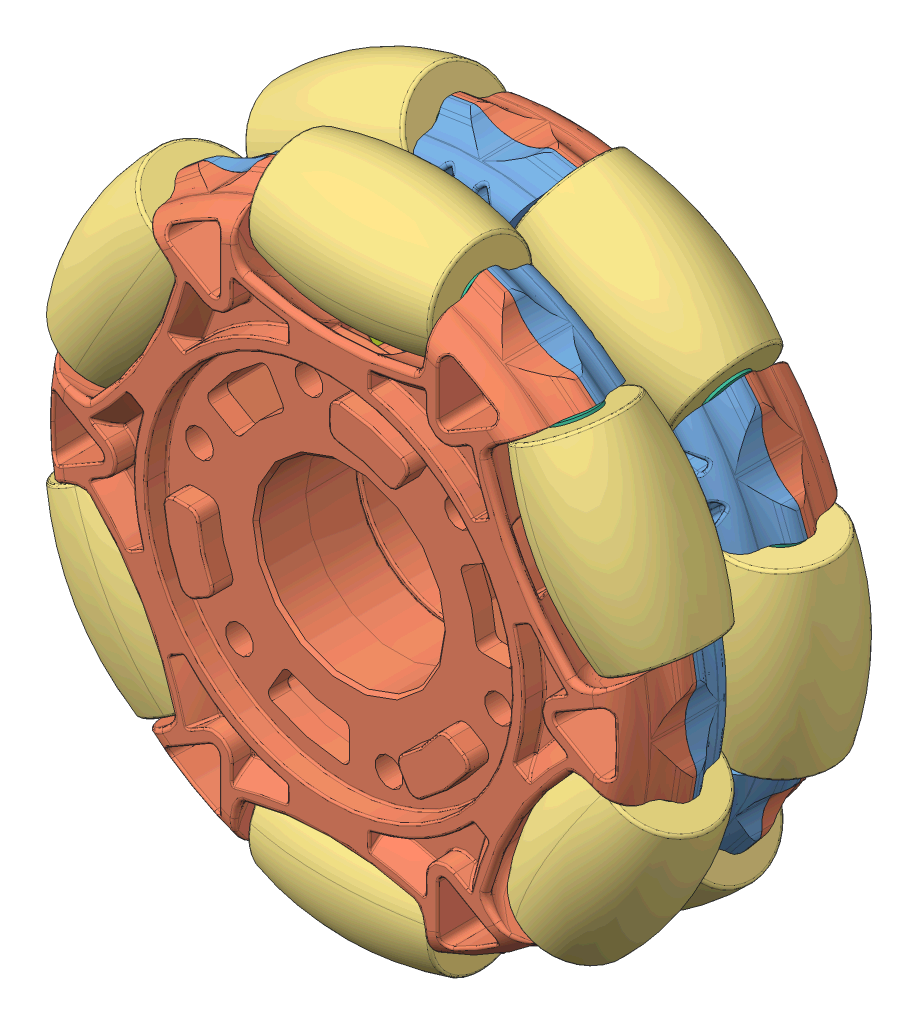
SolidWorks assembly 4_Omni-Directional_Wheel_v2_276-6194, configuration Default. Lengths in mm.
Overall size (126.87 125.33 42.82).
82 component instances, 8 part files, 0 mates.
Components (placement in the parent):
- 4_Omni-Directional_Wheel_v2_276-6194(2)-1: 4_Omni-Directional_Wheel_v2_276-6194(2) [Default] at origin size (126.87 125.33 42.82)
  - 217-6194-002 Rev5-1: 217-6194-002 Rev5 [Default] at origin size (94.42 94.42 19.26)
  - 217-6194-003 Rev8-1: 217-6194-003 Rev8 [Default] at (0 0 9.525) size (94.42 90.2 19.97)
  - 217-6194-003 Rev8-2: 217-6194-003 Rev8 [Default] at (0 0 -9.525) x (-0.866025 0.5 0) z (0 0 -1) size (94.42 90.2 19.97)
  - 217-6194-001 Rev3-1: 217-6194-001 Rev3 [Default] at (0 -40.8953 9.525) x (1 0 0) z (0 0.225507 0.974241) size (28 19.81 19.81)
  - 217-6194-008 Rev4-1: 217-6194-008 Rev4 [Default] at (0 -40.8953 9.525) x (0 0.977486 -0.211002) z (0 0.211002 0.977486) size (4.05 28 4.05)
  - 217-6194-004 Rev4-1: 217-6194-004 Rev4 [Default] at (0 -40.8953 9.525) size (33.5 3 3)
  - 217-2584-009 Rev1-1: 217-2584-009 Rev1 [Default] at (14.38 -40.8953 9.525) x (0 0.996349 0.085373) z (0 -0.085373 0.996349) size (7 0.38 7)
  - 217-2584-009 Rev1-2: 217-2584-009 Rev1 [Default] at (-14 -40.8953 9.525) x (0 0.996349 0.085373) z (0 -0.085373 0.996349) size (7 0.38 7)
  - 217-6194-004 Rev4-2: 217-6194-004 Rev4 [Default] at (-20.4477 -35.4164 -9.525) x (0.866025 -0.5 0) z (0 0 1) size (33.5 3 3)
  - 217-6194-008 Rev4-2: 217-6194-008 Rev4 [Default] at (-20.4477 -35.4164 -9.525) x (0.488743 0.846527 -0.211002) z (0.105501 0.182733 0.977486) size (4.05 28 4.05)
  - 217-6194-001 Rev3-2: 217-6194-001 Rev3 [Default] at (-20.4477 -35.4164 -9.525) x (0.866025 -0.5 0) z (0.112754 0.195295 0.974241) size (28 19.81 19.81)
  - 217-2584-009 Rev1-3: 217-2584-009 Rev1 [Default] at (-7.9942 -42.6064 -9.525) x (0.498175 0.862864 0.085373) z (-0.042686 -0.073935 0.996349) size (7 0.38 7)
  - 217-2584-009 Rev1-4: 217-2584-009 Rev1 [Default] at (-32.572 -28.4164 -9.525) x (0.498175 0.862864 0.085373) z (-0.042686 -0.073935 0.996349) size (7 0.38 7)
  - 217-6194-005 Rev1-1: 217-6194-005 Rev1 [Default] at (6.1631 -23.0011 0) x (0.707107 -0.707107 0) z (0.707107 0.707107 0) size (7.34 25.4 7.34)
  - 217-6194-005 Rev1-2: 217-6194-005 Rev1 [Default] at (23.0011 -6.1631 0) x (0.965926 0.258819 0) z (-0.258819 0.965926 0) size (7.34 25.4 7.34)
  - 217-6194-005 Rev1-3: 217-6194-005 Rev1 [Default] at (16.838 16.838 0) x (0.258819 0.965926 0) z (-0.965926 0.258819 0) size (7.34 25.4 7.34)
  - 217-6194-005 Rev1-4: 217-6194-005 Rev1 [Default] at (-6.1631 23.0011 0) x (-0.707107 0.707107 0) z (-0.707107 -0.707107 0) size (7.34 25.4 7.34)
  - 217-6194-005 Rev1-5: 217-6194-005 Rev1 [Default] at (-23.0011 6.1631 0) x (-0.965926 -0.258819 0) z (0.258819 -0.965926 0) size (7.34 25.4 7.34)
  - 217-6194-005 Rev1-6: 217-6194-005 Rev1 [Default] at (-16.838 -16.838 0) x (-0.258819 -0.965926 0) z (0.965926 -0.258819 0) size (7.34 25.4 7.34)
  - 217-2584-009 Rev1-5: 217-2584-009 Rev1 [Default] at (8.3233 -42.4164 -9.525) x (-0.498175 0.862864 0.085373) z (0.042686 -0.073935 0.996349) size (7 0.38 7)
  - 217-2584-009 Rev1-6: 217-2584-009 Rev1 [Default] at (40.8953 -14 -9.525) x (-0.996349 0 0.085373) z (0.085373 0 0.996349) size (7 0.38 7)
  - 217-2584-009 Rev1-7: 217-2584-009 Rev1 [Default] at (32.572 28.4164 -9.525) x (-0.498175 -0.862864 0.085373) z (0.042686 0.073935 0.996349) size (7 0.38 7)
  - 217-2584-009 Rev1-8: 217-2584-009 Rev1 [Default] at (-8.3233 42.4164 -9.525) x (0.498175 -0.862864 0.085373) z (-0.042686 0.073935 0.996349) size (7 0.38 7)
  - 217-2584-009 Rev1-9: 217-2584-009 Rev1 [Default] at (-40.8953 14 -9.525) x (0.996349 0 0.085373) z (-0.085373 0 0.996349) size (7 0.38 7)
  - 217-2584-009 Rev1-10: 217-2584-009 Rev1 [Default] at (32.9011 -28.2264 -9.525) x (-0.498175 0.862864 0.085373) z (0.042686 -0.073935 0.996349) size (7 0.38 7)
  - 217-2584-009 Rev1-11: 217-2584-009 Rev1 [Default] at (40.8953 14.38 -9.525) x (-0.996349 0 0.085373) z (0.085373 0 0.996349) size (7 0.38 7)
  - 217-2584-009 Rev1-12: 217-2584-009 Rev1 [Default] at (7.9942 42.6064 -9.525) x (-0.498175 -0.862864 0.085373) z (0.042686 0.073935 0.996349) size (7 0.38 7)
  - 217-2584-009 Rev1-13: 217-2584-009 Rev1 [Default] at (-32.9011 28.2264 -9.525) x (0.498175 -0.862864 0.085373) z (-0.042686 0.073935 0.996349) size (7 0.38 7)
  - 217-2584-009 Rev1-14: 217-2584-009 Rev1 [Default] at (-40.8953 -14.38 -9.525) x (0.996349 0 0.085373) z (-0.085373 0 0.996349) size (7 0.38 7)
  - 217-6194-001 Rev3-3: 217-6194-001 Rev3 [Default] at (20.4477 -35.4164 -9.525) x (0.866025 0.5 0) z (-0.112754 0.195295 0.974241) size (28 19.81 19.81)
  - 217-6194-001 Rev3-4: 217-6194-001 Rev3 [Default] at (40.8953 0 -9.525) x (0 1 0) z (-0.225507 0 0.974241) size (28 19.81 19.81)
  - 217-6194-001 Rev3-5: 217-6194-001 Rev3 [Default] at (20.4477 35.4164 -9.525) x (-0.866025 0.5 0) z (-0.112754 -0.195295 0.974241) size (28 19.81 19.81)
  - 217-6194-001 Rev3-6: 217-6194-001 Rev3 [Default] at (-20.4477 35.4164 -9.525) x (-0.866025 -0.5 0) z (0.112754 -0.195295 0.974241) size (28 19.81 19.81)
  - 217-6194-001 Rev3-7: 217-6194-001 Rev3 [Default] at (-40.8953 0 -9.525) x (0 -1 0) z (0.225507 0 0.974241) size (28 19.81 19.81)
  - 217-6194-008 Rev4-3: 217-6194-008 Rev4 [Default] at (20.4477 -35.4164 -9.525) x (-0.488743 0.846527 -0.211002) z (-0.105501 0.182733 0.977486) size (4.05 28 4.05)
  - 217-6194-008 Rev4-4: 217-6194-008 Rev4 [Default] at (40.8953 0 -9.525) x (-0.977486 0 -0.211002) z (-0.211002 0 0.977486) size (4.05 28 4.05)
  - 217-6194-008 Rev4-5: 217-6194-008 Rev4 [Default] at (20.4477 35.4164 -9.525) x (-0.488743 -0.846527 -0.211002) z (-0.105501 -0.182733 0.977486) size (4.05 28 4.05)
  - 217-6194-008 Rev4-6: 217-6194-008 Rev4 [Default] at (-20.4477 35.4164 -9.525) x (0.488743 -0.846527 -0.211002) z (0.105501 -0.182733 0.977486) size (4.05 28 4.05)
  - 217-6194-008 Rev4-7: 217-6194-008 Rev4 [Default] at (-40.8953 0 -9.525) x (0.977486 0 -0.211002) z (0.211002 0 0.977486) size (4.05 28 4.05)
  - 217-6194-004 Rev4-3: 217-6194-004 Rev4 [Default] at (20.4477 -35.4164 -9.525) x (0.866025 0.5 0) z (0 0 1) size (33.5 3 3)
  - 217-6194-004 Rev4-4: 217-6194-004 Rev4 [Default] at (40.8953 0 -9.525) x (0 1 0) z (0 0 1) size (33.5 3 3)
  - 217-6194-004 Rev4-5: 217-6194-004 Rev4 [Default] at (20.4477 35.4164 -9.525) x (-0.866025 0.5 0) z (0 0 1) size (33.5 3 3)
  - 217-6194-004 Rev4-6: 217-6194-004 Rev4 [Default] at (-20.4477 35.4164 -9.525) x (-0.866025 -0.5 0) z (0 0 1) size (33.5 3 3)
  - 217-6194-004 Rev4-7: 217-6194-004 Rev4 [Default] at (-40.8953 0 -9.525) x (0 -1 0) z (0 0 1) size (33.5 3 3)
  - 217-2584-009 Rev1-15: 217-2584-009 Rev1 [Default] at (28.4164 -32.572 9.525) x (-0.862864 0.498175 0.085373) z (0.073935 -0.042686 0.996349) size (7 0.38 7)
  - 217-2584-009 Rev1-16: 217-2584-009 Rev1 [Default] at (42.4164 8.3233 9.525) x (-0.862864 -0.498175 0.085373) z (0.073935 0.042686 0.996349) size (7 0.38 7)
  - 217-2584-009 Rev1-17: 217-2584-009 Rev1 [Default] at (14 40.8953 9.525) x (0 -0.996349 0.085373) z (0 0.085373 0.996349) size (7 0.38 7)
  - 217-2584-009 Rev1-18: 217-2584-009 Rev1 [Default] at (-28.4164 32.572 9.525) x (0.862864 -0.498175 0.085373) z (-0.073935 0.042686 0.996349) size (7 0.38 7)
  - 217-2584-009 Rev1-19: 217-2584-009 Rev1 [Default] at (-42.4164 -8.3233 9.525) x (0.862864 0.498175 0.085373) z (-0.073935 -0.042686 0.996349) size (7 0.38 7)
  - 217-2584-009 Rev1-20: 217-2584-009 Rev1 [Default] at (42.6064 -7.9942 9.525) x (-0.862864 0.498175 0.085373) z (0.073935 -0.042686 0.996349) size (7 0.38 7)
  - 217-2584-009 Rev1-21: 217-2584-009 Rev1 [Default] at (28.2264 32.9011 9.525) x (-0.862864 -0.498175 0.085373) z (0.073935 0.042686 0.996349) size (7 0.38 7)
  - 217-2584-009 Rev1-22: 217-2584-009 Rev1 [Default] at (-14.38 40.8953 9.525) x (0 -0.996349 0.085373) z (0 0.085373 0.996349) size (7 0.38 7)
  - 217-2584-009 Rev1-23: 217-2584-009 Rev1 [Default] at (-42.6064 7.9942 9.525) x (0.862864 -0.498175 0.085373) z (-0.073935 0.042686 0.996349) size (7 0.38 7)
  - 217-2584-009 Rev1-24: 217-2584-009 Rev1 [Default] at (-28.2264 -32.9011 9.525) x (0.862864 0.498175 0.085373) z (-0.073935 -0.042686 0.996349) size (7 0.38 7)
  - 217-6194-004 Rev4-8: 217-6194-004 Rev4 [Default] at (35.4164 -20.4477 9.525) x (0.5 0.866025 0) z (0 0 1) size (33.5 3 3)
  - 217-6194-004 Rev4-9: 217-6194-004 Rev4 [Default] at (35.4164 20.4477 9.525) x (-0.5 0.866025 0) z (0 0 1) size (33.5 3 3)
  - 217-6194-004 Rev4-10: 217-6194-004 Rev4 [Default] at (0 40.8953 9.525) x (-1 0 0) z (0 0 1) size (33.5 3 3)
  - 217-6194-004 Rev4-11: 217-6194-004 Rev4 [Default] at (-35.4164 20.4477 9.525) x (-0.5 -0.866025 0) z (0 0 1) size (33.5 3 3)
  - 217-6194-004 Rev4-12: 217-6194-004 Rev4 [Default] at (-35.4164 -20.4477 9.525) x (0.5 -0.866025 0) z (0 0 1) size (33.5 3 3)
  - 217-6194-008 Rev4-8: 217-6194-008 Rev4 [Default] at (35.4164 -20.4477 9.525) x (-0.846527 0.488743 -0.211002) z (-0.182733 0.105501 0.977486) size (4.05 28 4.05)
  - 217-6194-008 Rev4-9: 217-6194-008 Rev4 [Default] at (35.4164 20.4477 9.525) x (-0.846527 -0.488743 -0.211002) z (-0.182733 -0.105501 0.977486) size (4.05 28 4.05)
  - 217-6194-008 Rev4-10: 217-6194-008 Rev4 [Default] at (0 40.8953 9.525) x (0 -0.977486 -0.211002) z (0 -0.211002 0.977486) size (4.05 28 4.05)
  - 217-6194-008 Rev4-11: 217-6194-008 Rev4 [Default] at (-35.4164 20.4477 9.525) x (0.846527 -0.488743 -0.211002) z (0.182733 -0.105501 0.977486) size (4.05 28 4.05)
  - 217-6194-008 Rev4-12: 217-6194-008 Rev4 [Default] at (-35.4164 -20.4477 9.525) x (0.846527 0.488743 -0.211002) z (0.182733 0.105501 0.977486) size (4.05 28 4.05)
  - 217-6194-001 Rev3-8: 217-6194-001 Rev3 [Default] at (35.4164 -20.4477 9.525) x (0.5 0.866025 0) z (-0.195295 0.112754 0.974241) size (28 19.81 19.81)
  - 217-6194-001 Rev3-9: 217-6194-001 Rev3 [Default] at (35.4164 20.4477 9.525) x (-0.5 0.866025 0) z (-0.195295 -0.112754 0.974241) size (28 19.81 19.81)
  - 217-6194-001 Rev3-10: 217-6194-001 Rev3 [Default] at (0 40.8953 9.525) x (-1 0 0) z (0 -0.225507 0.974241) size (28 19.81 19.81)
  - 217-6194-001 Rev3-11: 217-6194-001 Rev3 [Default] at (-35.4164 20.4477 9.525) x (-0.5 -0.866025 0) z (0.195295 -0.112754 0.974241) size (28 19.81 19.81)
  - 217-6194-001 Rev3-12: 217-6194-001 Rev3 [Default] at (-35.4164 -20.4477 9.525) x (0.5 -0.866025 0) z (0.195295 0.112754 0.974241) size (28 19.81 19.81)
  - 217-4775-008 Rev1_90116A020-1: 217-4775-008 Rev1_90116A020 [Default] at (0 -40 -2.025) x (-0.89498 0.446105 0) z (0 0 -1) size (4.2 4.2 11.62)
  - 217-4775-008 Rev1_90116A020-2: 217-4775-008 Rev1_90116A020 [Default] at (20 -34.641 2.025) x (0.648091 0.761563 0) z (0 0 1) size (4.2 4.2 11.62)
  - 217-4775-008 Rev1_90116A020-3: 217-4775-008 Rev1_90116A020 [Default] at (40 0 2.025) x (-0.335487 0.942045 0) z (0 0 1) size (4.2 4.2 11.62)
  - 217-4775-008 Rev1_90116A020-4: 217-4775-008 Rev1_90116A020 [Default] at (20 34.641 2.025) x (-0.983578 0.180482 0) z (0 0 1) size (4.2 4.2 11.62)
  - 217-4775-008 Rev1_90116A020-5: 217-4775-008 Rev1_90116A020 [Default] at (-20 34.641 2.025) x (-0.648091 -0.761563 0) z (0 0 1) size (4.2 4.2 11.62)
  - 217-4775-008 Rev1_90116A020-6: 217-4775-008 Rev1_90116A020 [Default] at (-40 0 2.025) x (0.335487 -0.942045 0) z (0 0 1) size (4.2 4.2 11.62)
  - 217-4775-008 Rev1_90116A020-7: 217-4775-008 Rev1_90116A020 [Default] at (-20 -34.641 2.025) x (0.983578 -0.180482 0) z (0 0 1) size (4.2 4.2 11.62)
  - 217-4775-008 Rev1_90116A020-8: 217-4775-008 Rev1_90116A020 [Default] at (34.641 -20 -2.025) x (-0.833829 -0.552023 0) z (0 0 -1) size (4.2 4.2 11.62)
  - 217-4775-008 Rev1_90116A020-9: 217-4775-008 Rev1_90116A020 [Default] at (34.641 20 -2.025) x (0.061152 -0.998128 0) z (0 0 -1) size (4.2 4.2 11.62)
  - 217-4775-008 Rev1_90116A020-10: 217-4775-008 Rev1_90116A020 [Default] at (0 40 -2.025) x (0.89498 -0.446105 0) z (0 0 -1) size (4.2 4.2 11.62)
  - 217-4775-008 Rev1_90116A020-11: 217-4775-008 Rev1_90116A020 [Default] at (-34.641 20 -2.025) x (0.833829 0.552023 0) z (0 0 -1) size (4.2 4.2 11.62)
  - 217-4775-008 Rev1_90116A020-12: 217-4775-008 Rev1_90116A020 [Default] at (-34.641 -20 -2.025) x (-0.061152 0.998128 0) z (0 0 -1) size (4.2 4.2 11.62)
